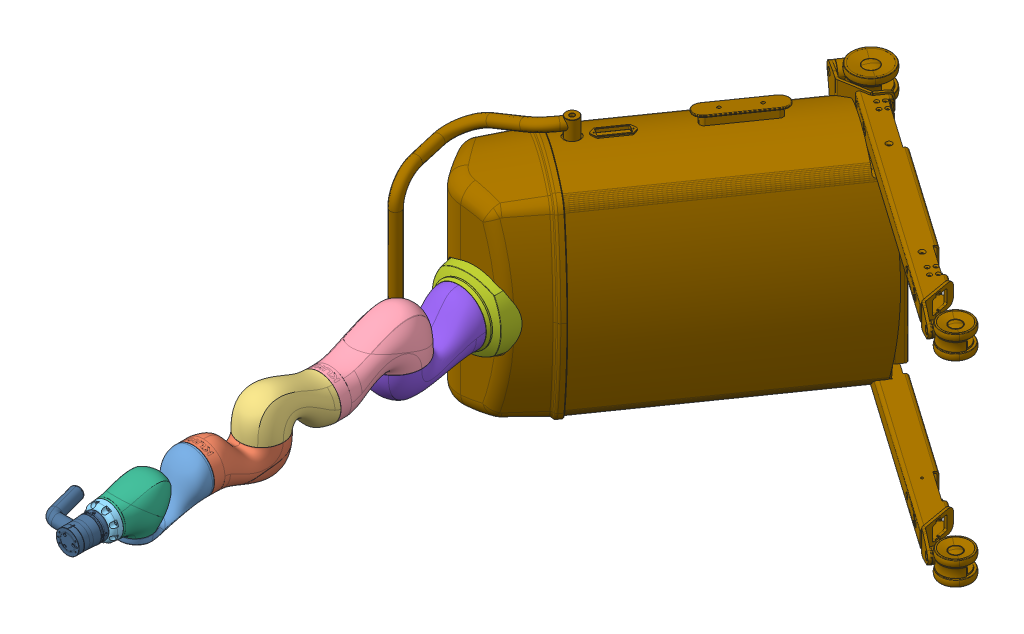
SolidWorks assembly lbrMed_withBaseLink, configuration Default. Lengths in mm.
Overall size (1621.06 766 2374.52).
10 component instances, 10 part files, 6 mates.
Components (placement in the parent):
- Wrist1_body-2: Wrist1_body [Default] at origin size (137.43 170.81 261.47)
- UpperArm_body-1: UpperArm_body [Default] at origin size (137.03 183.96 286.04)
- Elbow_body-1: Elbow_body [Default] at origin size (136.09 183.95 261.22)
- LowerArm_body-1: LowerArm_body [Default] at origin size (171.08 201.65 323.93)
- Wrist3_body-1: Wrist3_body [Default] at origin size (102.25 102.25 38.4)
- Wrist2_body-1: Wrist2_body [Default] at origin size (136.25 137.94 182.79)
- Base_body-1: Base_body [Default] at origin size (277.84 277.84 157.78)
- Shoulder_body-1: Shoulder_body [Default] at origin size (171.08 202.96 299.34)
- only_platform-1: only_platform [Default] at (515.1468 0 -732.7058) x (-0.819152 0 -0.573576) z (0 1 0) size (1151.95 1181.08 766)
- only_link-1: only_link [Default] at (515.1468 0 -732.7058) x (-0.819152 0 -0.573576) z (0 1 0) size (227.18 131.55 78.48)
Mates (geometry in assembly coordinates):
- Concentric1: concentric: cylinder of Base_body-1 through (84.8528 84.8528 0) axis (0 0 1) radius 5; cylinder of only_platform-1 through (84.8528 84.8528 -125.779) axis (0 0 1) radius 5.25
- Concentric2: concentric: cylinder of Base_body-1 through (84.8528 -84.8528 0) axis (0 0 1) radius 5; cylinder of only_platform-1 through (84.8528 -84.8528 -125.779) axis (0 0 1) radius 5.25
- Coincident1: coincident anti-aligned: plane of Base_body-1 through (0 0 3) normal (0 0 -1); plane of only_platform-1 through (127.5 127.5 3) normal (0 0 1)
- Concentric3: concentric: cylinder of Wrist3_body-1 through (-9.7581 9.7581 1289.3) axis (0 0 1) radius 3.2; cylinder of only_link-1 through (-9.7581 9.7581 1374.0312) axis (0 0 -1) radius 3.2
- Concentric4: concentric: cylinder of Wrist3_body-1 through (9.7581 -9.7581 1289.3) axis (0 0 1) radius 3.2; cylinder of only_link-1 through (9.7581 -9.7581 1305.98) axis (0 0 -1) radius 3.2
- Coincident2: coincident anti-aligned: plane of Wrist3_body-1 through (0 30.5 1306) normal (0 0 1); plane of only_link-1 through (0 0 1306) normal (0 0 -1)
